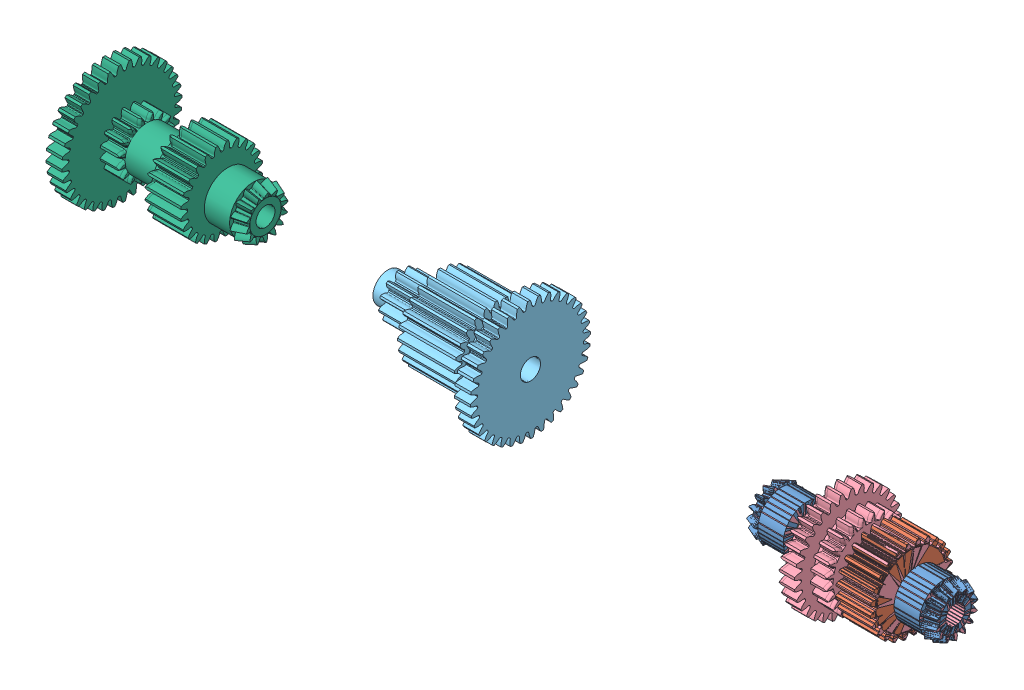
SolidWorks assembly 齿轮打印, configuration 默认. Lengths in mm.
Overall size (137.47 19 19).
30 component instances, 20 part files, 33 mates.
Components (placement in the parent):
- 前后传动锥齿14-1: 前后传动锥齿14 [GB - Straight bevel pinion 0.5M14PT 42GT 20PA 2FW ---14O7.5H14MD3.0N] at (-15.0061 18.2039 363.5733) x (-1 0 0) z (0 0.771671 -0.636022) size (6.25 8.01 8.21)
- 圆柱齿轮24×5-1: 圆柱齿轮24×5 [默认] at (5.4939 18.2039 363.5733) x (0 0.042161 0.999111) z (-1 0 0) size (12.93 12.93 5.5)
- 前后传动锥齿14-2: 前后传动锥齿14 [GB - Straight bevel pinion 0.5M14PT 42GT 20PA 2FW ---14O7.5H14MD3.0N] at (10.4939 18.2039 363.5733) x (1 0 0) z (0 0.882489 -0.470333) size (6.25 8.01 8.21)
- 装配体齿轮连接件-4: 装配体齿轮连接件 [默认] at (-0.0061 18.2039 363.5733) x (0 -0.109824 0.993951) z (-1 0 0) size (3.85 3.85 1)
- 电机固定传动齿轮3mm-1: 电机固定传动齿轮3mm [默认] at (11.1867 17.3162 364.6735) x (0 -0.94948 -0.313826) z (-1 0 0) size (18.79 18.79 9) (hidden)
  - 传动齿轮24x3-1: 传动齿轮24x3 [默认] at (-0.4976 -1.3232 12.6928) x (0.102928 -0.994689 0) z (0 0 1) size (13.09 13.09 3.5)
  - 圆柱齿轮32×3-1: 圆柱齿轮32×3 [默认] at (-0.4976 -1.3232 15.6928) x (-0.102928 0.994689 0) z (0 0 1) size (17.12 17.12 2.51)
  - 传动齿轮12x3-1: 传动齿轮12x3 [默认] at (-0.4976 -1.3232 18.1928) x (-0.102928 0.994689 0) z (0 0 1) size (6.83 6.83 3)
- 装配体齿轮连接件-11: 装配体齿轮连接件 [默认] at (6.4939 18.2039 363.5733) x (0 -0.109824 0.993951) z (-1 0 0) size (3.85 3.85 1)
- 装配体齿轮连接件-5: 装配体齿轮连接件 [默认] at (-10.0061 18.2039 363.5733) x (0 -0.109824 0.993951) z (-1 0 0) size (3.85 3.85 1)
- 电机滑动传动齿轮2mm-1: 电机滑动传动齿轮2mm [默认] at (-120.926 22.6637 365.7612) x (0.069163 0.019015 0.997424) z (0.96378 -0.259418 -0.061884) size (13.39 14.37 17.14) (hidden)
  - 传动齿轮24x2-1: 传动齿轮24x2 [默认] at (-1.0598 -0.2692 18.1158) x (-0.997571 -0.025895 0.064667) z (-0.069163 0.257573 -0.96378) size (13.09 13.09 11.75) (hidden)
  - 圆柱齿轮16×2-1: 圆柱齿轮16×2 [默认] at (-2.0799 3.53 3.9) x (-0.997571 -0.025895 0.064667) z (0.069163 -0.257573 0.96378) size (9.04 9.04 3.01) (hidden)
  - 齿轮32x24-1: 齿轮32x24 [默认] at origin size (13.39 14.37 17.14)
- 电机垂直传动齿轮2mm-1: 电机垂直传动齿轮2mm [默认] at (-128.7661 18.2039 363.5733) x (-1 0 0) z (0 -0.381207 -0.92449) size (5.5 18.97 18.97) (hidden)
  - 传动齿轮12x2-1: 传动齿轮12x2 [默认] at (-4.0458 0 0) x (0 0.164744 0.986336) z (-1 0 0) size (6.83 6.83 3) (hidden)
  - 36锥齿轮零件-1: 36锥齿轮零件 [默认] at origin size (5.5 18.97 18.97)
  - 圆柱齿轮36×2-1: 圆柱齿轮36×2 [默认] at (-7.0458 0 0) x (0 0.164744 0.986336) z (-1 0 0) size (18.96 18.96 2.5) (hidden)
- 电机传动齿轮3mm-1: 电机传动齿轮3mm [默认] at (-37.9532 16.5577 366.2861) x (0 -0.617758 0.786368) z (-1 0 0) size (18.99 18.99 14.5) (hidden)
  - 传动齿轮36x3-1: 传动齿轮36x3 [默认] at (-3.1503 -0.3813 16.7455) x (0.028836 -0.999584 0) z (0 0 1) size (18.96 18.96 5.5) (hidden)
  - 电机传动3mm-1: 电机传动3mm [默认] at origin size (18.99 18.99 14.5)
  - 圆柱齿轮24×3滑-1: 圆柱齿轮24×3滑 [默认] at (-3.1503 -0.3813 22.2455) x (0.028836 -0.999584 0) z (0 0 1) size (12.93 12.93 9) (hidden)
- 装配体齿轮连接件32-1: 装配体齿轮连接件32 [默认] at (-70.1987 18.2039 363.5733) x (0 -0.529835 -0.848101) z (1 0 0) size (4 4 1) (hidden)
- 前后传动锥齿14-4: 前后传动锥齿14 [GB - Straight bevel pinion 0.5M14PT 42GT 20PA 2FW ---14O7.5H14MD3.0N] at (-98.4704 18.2039 363.5733) x (1 0 0) z (0 0.882489 -0.470333) size (6.25 8.01 8.21) (hidden)
- 装配体齿轮连接件-9: 装配体齿轮连接件 [默认] at (-102.4704 18.2039 363.5733) x (0 -0.109824 0.993951) z (-1 0 0) size (3.85 3.85 1) (hidden)
- 装配体齿轮连接件-10: 装配体齿轮连接件 [默认] at (-118.2204 18.2039 363.5733) x (0 -0.109824 0.993951) z (-1 0 0) size (3.85 3.85 1) (hidden)
- 齿轮打印305-1: 齿轮打印305 [默认] at (0 0 73.9459) size (30.01 17.14 17.14)
- 齿轮打印32-1: 齿轮打印32 [默认] at origin size (22.5 19 19)
- 齿轮打印22-1: 齿轮打印22 [默认] at origin size (28.5 19 19)
- 电机齿轮12-1: 电机齿轮12 [默认] at (-75.1987 18.2039 363.5733) x (0 -0.116024 -0.993246) z (1 0 0) size (6.83 6.83 7) (hidden)
Mates (geometry in assembly coordinates):
- 平行1: parallel aligned: plane of 电机滑动传动齿轮2mm-1/齿轮32x24-1 through (-103.4704 18.2039 363.5733) normal (1 0 0); plane of 电机传动齿轮3mm-1/电机传动3mm-1 through (-60.1987 18.2039 363.5733) normal (1 0 0)
- 同心1: concentric anti-aligned: cylinder of 电机固定传动齿轮3mm-1/齿轮24x32-1 through (0.9939 18.2039 363.5733) axis (1 0 0) radius 1.525; cylinder of 电机传动齿轮3mm-1/电机传动3mm-1 through (-54.6977 18.2039 363.5733) axis (-1 0 0) radius 1.6
- 同心2: concentric anti-aligned: cylinder of 圆柱齿轮24×5-1 through (5.4949 18.2039 363.5733) axis (-1 0 0) radius 1.525; cylinder of 电机滑动传动齿轮2mm-1/齿轮32x24-1 through (-115.2214 18.2039 363.5733) axis (1 0 0) radius 1.1
- 同心3: concentric anti-aligned: cylinder of 电机垂直传动齿轮2mm-1/36锥齿轮零件-1 through (-124.7214 18.2039 363.5733) axis (1 0 0) radius 1.1; cylinder of 圆柱齿轮24×5-1 through (5.4949 18.2039 363.5733) axis (-1 0 0) radius 1.525
- 同心4: concentric aligned: cylinder of 圆柱齿轮24×5-1 through (5.4949 18.2039 363.5733) axis (-1 0 0) radius 1.525; cylinder of 电机传动齿轮3mm-1/电机传动3mm-1 through (-54.6977 18.2039 363.5733) axis (-1 0 0) radius 1.6
- 同心11: concentric aligned: cylinder of 电机垂直传动齿轮2mm-1/36锥齿轮零件-1 through (-124.7214 18.2039 363.5733) axis (1 0 0) radius 1.1; cylinder of 装配体齿轮连接件-4 through (-1.0061 18.2039 363.5733) axis (1 0 0) radius 1.525
- 同心12: concentric aligned: cylinder of 电机垂直传动齿轮2mm-1/36锥齿轮零件-1 through (-124.7214 18.2039 363.5733) axis (1 0 0) radius 1.1; cylinder of 装配体齿轮连接件-5 through (-11.0061 18.2039 363.5733) axis (1 0 0) radius 1.525
- 重合5: coincident anti-aligned: plane of 电机固定传动齿轮3mm-1/齿轮24x32-1 through (-10.0061 18.2039 363.5733) normal (-1 0 0); plane of 装配体齿轮连接件-5 through (-10.0061 18.2039 363.5733) normal (1 0 0)
- 重合6: coincident anti-aligned: plane of 前后传动锥齿14-1 through (-11.0061 18.2039 363.5733) normal (1 0 0); plane of 装配体齿轮连接件-5 through (-11.0061 18.2039 363.5733) normal (-1 0 0)
- 重合7: coincident anti-aligned: plane of 圆柱齿轮24×5-1 through (-0.0061 18.2039 363.5733) normal (-1 0 0); plane of 装配体齿轮连接件-4 through (-0.0061 18.2039 363.5733) normal (1 0 0)
- 重合8: coincident anti-aligned: plane of 电机固定传动齿轮3mm-1/齿轮24x32-1 through (-1.0061 18.2039 363.5733) normal (1 0 0); plane of 装配体齿轮连接件-4 through (-1.0061 18.2039 363.5733) normal (-1 0 0)
- 同心13: concentric anti-aligned: cylinder of 电机传动齿轮3mm-1/电机传动3mm-1 through (-75.9266 18.2039 363.5733) axis (1 0 0) radius 4.5; cylinder of 装配体齿轮连接件32-1 through (-69.1987 18.2039 363.5733) axis (-1 0 0) radius 2
- 重合11: coincident anti-aligned: plane of 电机传动齿轮3mm-1/电机传动3mm-1 through (-69.1987 18.2039 363.5733) normal (-1 0 0); plane of 装配体齿轮连接件32-1 through (-69.1987 18.2039 363.5733) normal (1 0 0)
- 同心15: concentric aligned: cylinder of 前后传动锥齿14-4 through (-102.4704 18.2039 363.5733) axis (1 0 0) radius 3.75; cylinder of 装配体齿轮连接件-9 through (-103.4704 18.2039 363.5733) axis (1 0 0) radius 1.925
- 重合15: coincident anti-aligned: plane of 前后传动锥齿14-4 through (-102.4704 18.2039 363.5733) normal (-1 0 0); plane of 装配体齿轮连接件-9 through (-102.4704 18.2039 363.5733) normal (1 0 0)
- 同心17: concentric aligned: cylinder of 电机滑动传动齿轮2mm-1/齿轮32x24-1 through (-115.2204 18.2039 363.5733) axis (1 0 0) radius 3.5; cylinder of 前后传动锥齿14-4 through (-102.4704 18.2039 363.5733) axis (1 0 0) radius 3.75
- 重合16: coincident anti-aligned: plane of 电机滑动传动齿轮2mm-1/齿轮32x24-1 through (-103.4704 18.2039 363.5733) normal (1 0 0); plane of 装配体齿轮连接件-9 through (-103.4704 18.2039 363.5733) normal (-1 0 0)
- 同心18: concentric aligned: cylinder of 电机滑动传动齿轮2mm-1/齿轮32x24-1 through (-115.2204 18.2039 363.5733) axis (1 0 0) radius 3.5; cylinder of 装配体齿轮连接件-10 through (-119.2204 18.2039 363.5733) axis (1 0 0) radius 1.925
- 重合17: coincident anti-aligned: plane of 电机滑动传动齿轮2mm-1/齿轮32x24-1 through (-118.2204 18.2039 363.5733) normal (-1 0 0); plane of 装配体齿轮连接件-10 through (-118.2204 18.2039 363.5733) normal (1 0 0)
- 重合18: coincident anti-aligned: plane of 电机垂直传动齿轮2mm-1/36锥齿轮零件-1 through (-119.2204 18.2039 363.5733) normal (1 0 0); plane of 装配体齿轮连接件-10 through (-119.2204 18.2039 363.5733) normal (-1 0 0)
- 同心20: concentric anti-aligned: cylinder of 圆柱齿轮24×5-1 through (5.4949 18.2039 363.5733) axis (-1 0 0) radius 1.525; cylinder of 装配体齿轮连接件-11 through (5.4939 18.2039 363.5733) axis (1 0 0) radius 1.525
- 重合21: coincident anti-aligned: plane of 前后传动锥齿14-2 through (6.4939 18.2039 363.5733) normal (-1 0 0); plane of 装配体齿轮连接件-11 through (6.4939 18.2039 363.5733) normal (1 0 0)
- 重合22: coincident anti-aligned: plane of 圆柱齿轮24×5-1 through (5.4939 18.2039 363.5733) normal (1 0 0); plane of 装配体齿轮连接件-11 through (5.4939 18.2039 363.5733) normal (-1 0 0)
- 在位2: in place: plane of ? through (0 0 0) normal (0 0 1); moOrthogonalPlaneRef_w of ? through (0 0 0) normal (0 1 0); plane of ? through (0 0 0) normal (1 0 0); unknown of ?
- 重合26: coincident aligned: 
- 重合27: coincident aligned: plane of 零件2^齿轮打印-1 through (0 0 0) normal (0 1 0)
- 重合28: coincident anti-aligned: plane of 零件2^齿轮打印-1 through (0 0 0) normal (1 0 0)
- 在位3: in place: plane of ? through (0 0 0) normal (0 0 1); plane of ? through (0 0 0) normal (0 1 0); plane of ? through (0 0 0) normal (1 0 0); unknown of ?
- 重合29: coincident aligned: 
- 重合30: coincident aligned: plane of 零件3^齿轮打印-1 through (0 0 0) normal (0 1 0)
- 重合31: coincident anti-aligned: plane of 零件3^齿轮打印-1 through (0 0 0) normal (1 0 0)
- 重合23: coincident anti-aligned: plane of 装配体齿轮连接件32-1 through (-70.1987 18.2039 363.5733) normal (-1 0 0); plane of 电机齿轮12-1 through (-70.1987 18.2039 363.5733) normal (1 0 0)
- 同心21: concentric anti-aligned: cylinder of 装配体齿轮连接件32-1 through (-69.1987 18.2039 363.5733) axis (-1 0 0) radius 2; cylinder of 电机齿轮12-1 through (-77.1987 18.2039 363.5733) axis (1 0 0) radius 2.38
